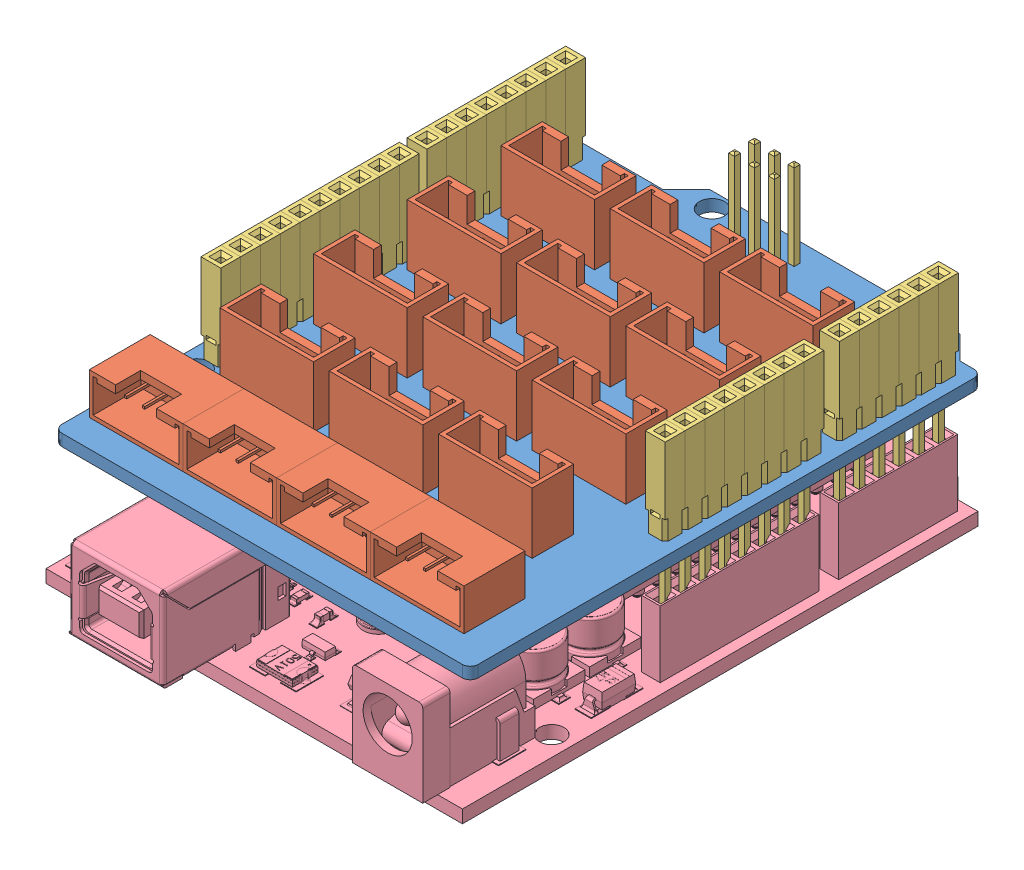
SolidWorks assembly Ensamblaje4, configuration Predeterminado. Lengths in mm.
Overall size (53.48 30.58 75.74).
62 component instances, 4 part files, 6 mates.
Components (placement in the parent):
- Base Shield-1: Base Shield [Défaut] at (-27.6351 -53.574 -33.8465) x (0 0 -1) z (0 1 0) size (68.53 53.3 23.9)
  - Plaque support BSG-1: Plaque support BSG [Défaut] at (1.2775 -1.1272 67.25) size (68.53 53.3 1.5)
  - Grove Connecteur BSG-1: Grove Connecteur BSG [Défaut] at (18.4925 14.5228 78) x (0 0 -1) z (0 -1 0) size (7.8 5.3 12)
  - Grove Connecteur BSG-2: Grove Connecteur BSG [Défaut] at (18.4925 0.5228 78) x (0 0 -1) z (0 -1 0) size (7.8 5.3 12)
  - Grove Connecteur BSG-3: Grove Connecteur BSG [Défaut] at (18.4925 -13.4772 78) x (0 0 -1) z (0 -1 0) size (7.8 5.3 12)
  - Grove Connecteur BSG-4: Grove Connecteur BSG [Défaut] at (6.4925 14.5228 78) x (0 0 -1) z (0 -1 0) size (7.8 5.3 12)
  - Grove Connecteur BSG-5: Grove Connecteur BSG [Défaut] at (6.4925 0.5228 78) x (0 0 -1) z (0 -1 0) size (7.8 5.3 12)
  - Grove Connecteur BSG-6: Grove Connecteur BSG [Défaut] at (6.4925 -13.4772 78) x (0 0 -1) z (0 -1 0) size (7.8 5.3 12)
  - Grove Connecteur BSG-7: Grove Connecteur BSG [Défaut] at (-5.5075 14.5228 78) x (0 0 -1) z (0 -1 0) size (7.8 5.3 12)
  - Grove Connecteur BSG-8: Grove Connecteur BSG [Défaut] at (-5.5075 0.5228 78) x (0 0 -1) z (0 -1 0) size (7.8 5.3 12)
  - Grove Connecteur BSG-9: Grove Connecteur BSG [Défaut] at (-5.5075 -13.4772 78) x (0 0 -1) z (0 -1 0) size (7.8 5.3 12)
  - Grove Connecteur BSG-10: Grove Connecteur BSG [Défaut] at (-17.5075 14.5228 78) x (0 0 -1) z (0 -1 0) size (7.8 5.3 12)
  - Grove Connecteur BSG-11: Grove Connecteur BSG [Défaut] at (-17.5075 0.5228 78) x (0 0 -1) z (0 -1 0) size (7.8 5.3 12)
  - Grove Connecteur BSG-12: Grove Connecteur BSG [Défaut] at (-17.5075 -13.4772 78) x (0 0 -1) z (0 -1 0) size (7.8 5.3 12)
  - Grove Connecteur BSG-13: Grove Connecteur BSG [Défaut] at (-30.9375 18.5228 68) x (1 0 0) z (0 -1 0) size (7.8 5.3 12)
  - Grove Connecteur BSG-14: Grove Connecteur BSG [Défaut] at (-30.9375 6.5228 68) x (1 0 0) z (0 -1 0) size (7.8 5.3 12)
  - Grove Connecteur BSG-15: Grove Connecteur BSG [Défaut] at (-30.9375 -5.4772 68) x (1 0 0) z (0 -1 0) size (7.8 5.3 12)
  - Grove Connecteur BSG-16: Grove Connecteur BSG [Défaut] at (-30.9375 -17.4772 68) x (1 0 0) z (0 -1 0) size (7.8 5.3 12)
  - Barre_8pins_bs_bleu-1: Barre_8pins_bs_bleu [Défaut] at (5.8965 28.1355 69.3083) x (0 1 0) z (1 0 0) size (2.54 23.88 20.32)
    - Pin_bs_bleu-1: Pin_bs_bleu [Défaut] at (-5.3827 -0.5583 23.876) size (2.54 23.88 2.54)
    - Pin_bs_bleu-2: Pin_bs_bleu [Défaut] at (-5.3827 -0.5583 21.336) size (2.54 23.88 2.54)
    - Pin_bs_bleu-3: Pin_bs_bleu [Défaut] at (-5.3827 -0.5583 18.796) size (2.54 23.88 2.54)
    - Pin_bs_bleu-4: Pin_bs_bleu [Défaut] at (-5.3827 -0.5583 16.256) size (2.54 23.88 2.54)
    - Pin_bs_bleu-5: Pin_bs_bleu [Défaut] at (-5.3827 -0.5583 13.716) size (2.54 23.88 2.54)
    - Pin_bs_bleu-6: Pin_bs_bleu [Défaut] at (-5.3827 -0.5583 11.176) size (2.54 23.88 2.54)
    - Pin_bs_bleu-7: Pin_bs_bleu [Défaut] at (-5.3827 -0.5583 8.636) size (2.54 23.88 2.54)
    - Pin_bs_bleu-8: Pin_bs_bleu [Défaut] at (-5.3827 -0.5583 6.096) size (2.54 23.88 2.54)
  - Barre_8pins_bs_bleu-2: Barre_8pins_bs_bleu [Défaut] at (-11.3435 -19.6245 69.3083) x (0 1 0) z (1 0 0) size (2.54 23.88 20.32)
    - Pin_bs_bleu-1: Pin_bs_bleu [Défaut] at (-5.3827 -0.5583 23.876) size (2.54 23.88 2.54)
    - Pin_bs_bleu-2: Pin_bs_bleu [Défaut] at (-5.3827 -0.5583 21.336) size (2.54 23.88 2.54)
    - Pin_bs_bleu-3: Pin_bs_bleu [Défaut] at (-5.3827 -0.5583 18.796) size (2.54 23.88 2.54)
    - Pin_bs_bleu-4: Pin_bs_bleu [Défaut] at (-5.3827 -0.5583 16.256) size (2.54 23.88 2.54)
    - Pin_bs_bleu-5: Pin_bs_bleu [Défaut] at (-5.3827 -0.5583 13.716) size (2.54 23.88 2.54)
    - Pin_bs_bleu-6: Pin_bs_bleu [Défaut] at (-5.3827 -0.5583 11.176) size (2.54 23.88 2.54)
    - Pin_bs_bleu-7: Pin_bs_bleu [Défaut] at (-5.3827 -0.5583 8.636) size (2.54 23.88 2.54)
    - Pin_bs_bleu-8: Pin_bs_bleu [Défaut] at (-5.3827 -0.5583 6.096) size (2.54 23.88 2.54)
  - Barre_10pins_bs_bleu-1: Barre_10pins_bs_bleu [Défaut] at (-15.4235 28.6772 68.4619) x (0 1 0) z (1 0 0) size (2.54 23.88 25.4)
    - Pin_bs_bleu-1: Pin_bs_bleu [Défaut] at (-5.9244 0.2881 23.876) size (2.54 23.88 2.54)
    - Pin_bs_bleu-2: Pin_bs_bleu [Défaut] at (-5.9244 0.2881 21.336) size (2.54 23.88 2.54)
    - Pin_bs_bleu-3: Pin_bs_bleu [Défaut] at (-5.9244 0.2881 18.796) size (2.54 23.88 2.54)
    - Pin_bs_bleu-4: Pin_bs_bleu [Défaut] at (-5.9244 0.2881 16.256) size (2.54 23.88 2.54)
    - Pin_bs_bleu-5: Pin_bs_bleu [Défaut] at (-5.9244 0.2881 13.716) size (2.54 23.88 2.54)
    - Pin_bs_bleu-6: Pin_bs_bleu [Défaut] at (-5.9244 0.2881 11.176) size (2.54 23.88 2.54)
    - Pin_bs_bleu-7: Pin_bs_bleu [Défaut] at (-5.9244 0.2881 8.636) size (2.54 23.88 2.54)
    - Pin_bs_bleu-8: Pin_bs_bleu [Défaut] at (-5.9244 0.2881 6.096) size (2.54 23.88 2.54)
    - Pin_bs_bleu-9: Pin_bs_bleu [Défaut] at (-5.9244 0.2881 3.556) size (2.54 23.88 2.54)
    - Pin_bs_bleu-10: Pin_bs_bleu [Défaut] at (-5.9244 0.2881 1.016) size (2.54 23.88 2.54)
  - Barre_6pins_bs_bleu-1: Barre_6pins_bs_bleu [Défaut] at (40.9485 -29.1712 69.6807) x (0 -1 0) z (-1 0 0) size (2.54 23.88 15.24)
    - Pin_bs_bleu-1: Pin_bs_bleu [Défaut] at (-4.164 -0.9307 23.876) size (2.54 23.88 2.54)
    - Pin_bs_bleu-2: Pin_bs_bleu [Défaut] at (-4.164 -0.9307 21.336) size (2.54 23.88 2.54)
    - Pin_bs_bleu-3: Pin_bs_bleu [Défaut] at (-4.164 -0.9307 18.796) size (2.54 23.88 2.54)
    - Pin_bs_bleu-4: Pin_bs_bleu [Défaut] at (-4.164 -0.9307 16.256) size (2.54 23.88 2.54)
    - Pin_bs_bleu-5: Pin_bs_bleu [Défaut] at (-4.164 -0.9307 13.716) size (2.54 23.88 2.54)
    - Pin_bs_bleu-6: Pin_bs_bleu [Défaut] at (-4.164 -0.9307 11.176) size (2.54 23.88 2.54)
  - Barre_2x3pins_bs_bleu-1: Barre_2x3pins_bs_bleu [Défaut] at (32.0268 25.4488 65.8454) x (-1 0 0) z (0 -1 0) size (5.08 23.88 7.62)
    - Pin_bs_bleu-1: Pin_bs_bleu [Défaut] at (1.7942 -1.4046 23.876) size (2.54 23.88 2.54)
    - Pin_bs_bleu-2: Pin_bs_bleu [Défaut] at (-0.7458 -1.4046 23.876) size (2.54 23.88 2.54)
    - Pin_bs_bleu-3: Pin_bs_bleu [Défaut] at (1.7942 -1.4046 26.416) size (2.54 23.88 2.54)
    - Pin_bs_bleu-4: Pin_bs_bleu [Défaut] at (-0.7458 -1.4046 26.416) size (2.54 23.88 2.54)
    - Pin_bs_bleu-5: Pin_bs_bleu [Défaut] at (1.7942 -1.4046 28.956) size (2.54 23.88 2.54)
    - Pin_bs_bleu-6: Pin_bs_bleu [Défaut] at (-0.7458 -1.4046 28.956) size (2.54 23.88 2.54)
- Arduino Uno(1)-1: Arduino Uno(1) [Default] at origin size (53.34 15.25 74.93)
Mates (geometry in assembly coordinates):
- Coincidente1: coordinate: point of Arduino Uno(1)-1
- Paralelo1: parallel: plane of Base Shield-1/Plaque support BSG-1 through (-0.8578 14.1681 -1.859) normal (0 -1 0); plane of Arduino Uno(1)-1 through (0 0 0) normal (0 1 0)
- Paralelo2: parallel: cylinder of Base Shield-1/Plaque support BSG-1 through (-7.5278 15.6681 -67.389) axis (0 -1 0) radius 1.61; cylinder of Arduino Uno(1)-1 through (-7.62 -1.65 -66.04) axis (0 1 0) radius 1.5875
- Paralelo3: parallel: cylinder of Base Shield-1/Plaque support BSG-1 through (-7.5278 15.6681 -67.389) axis (0 -1 0) radius 1.61; cylinder of Arduino Uno(1)-1 through (-7.62 -1.65 -66.04) axis (0 1 0) radius 1.5875
- Coincidente3: coincident: plane of Base Shield-1/Barre_8pins_bs_bleu-1/Pin_bs_bleu-1 through (-50.0068 2.476 -64) normal (0 0 -1); plane of Arduino Uno(1)-1 through (-51.3 3.51 -64) normal (0 0 1)
- Coincidente4: coincident anti-aligned: plane of Base Shield-1/Barre_2x3pins_bs_bleu-1/Pin_bs_bleu-6 through (-22.8578 2.5 -65.984) normal (0 -1 0); plane of Arduino Uno(1)-1 through (-26.12 2.5 -62.91) normal (0 1 0)
